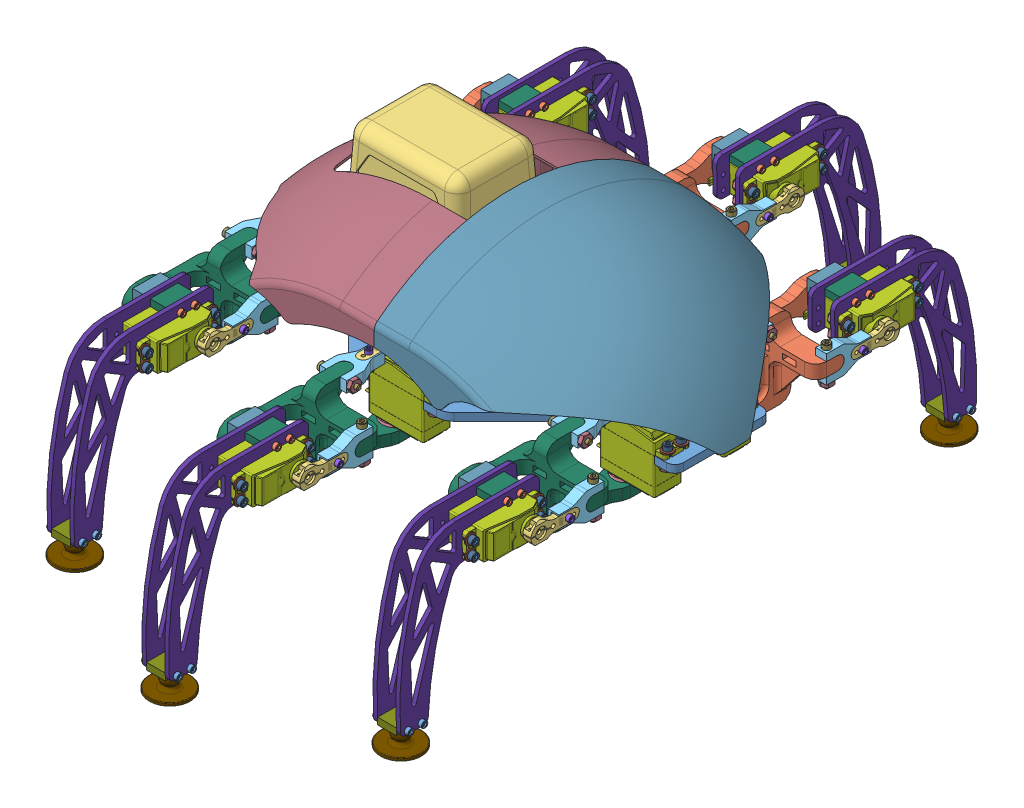
SolidWorks assembly Hexapod_(Small), configuration Défaut. Lengths in mm. (continued)
Components (placement in the parent): (continued)
- Foot+Femur_(Mirror)-8: Foot+Femur_(Mirror) [Défaut] at (-254.8 -28 0) x (0 0 1) z (-1 0 0) size (215.83 135.72 63.38)
  - Femur_(Mirror)-1: Femur_(Mirror) [Défaut] at origin size (137.38 61.64 60.79) (flexible)
    - Joint_(Femur_to_tibia)_(Mirror)-2: Joint_(Femur_to_tibia)_(Mirror) [Défaut] at (-66.2306 29.5 32.9516) x (0.999952 0 0.00979) z (-0.00979 0 0.999952) size (122 58.8 58.8)
    - Horn-4: Horn [Défaut] at (-10.2 48.8 30.1) x (-0.999952 0 -0.00979) z (0 1 0) size (35.39 15.87 6)
    - Bearing_mount_(Femur)-2: Bearing_mount_(Femur) [Default] at (2.5 22 30.1) x (1 0 0) z (0 -1 0) size (35.3 20.2 31)
    - Horn_attachment-4: Horn_attachment [Défaut] at (-38.1987 44.8 29.8259) x (0.999952 0 0.00979) z (0 1 0) size (33 20 8)
    - Bearing-4: Bearing [Default] at (-10.2 -6.7498 30.1) x (0.165905 0 -0.986142) z (0.986142 0 0.165905) size (13.87 4.75 13.87)
    - DS3225MG-4: DS3225MG [Default] at (-10.2 45.8 30.1) x (0 0 -1) z (0 1 0) size (57.25 20.4 45.91)
    - HX-SHCS 0.112-40x0.4375x0.4375-N-1: HX-SHCS 0.112-40x0.4375x0.4375-N [HX-SHCS 0.112-40x0.4375x0.4375-N] at (-30.199 51.6448 29.9042) x (0 -1 0) z (-0.508455 0 0.861089) size (13.96 4.65 4.65)
    - MSHXNUT 0.112-40-D-N-1: MSHXNUT 0.112-40-D-N [MSHXNUT 0.112-40-D-N] at (-30.199 40.8 29.9042) x (-0.491498 0 -0.870879) z (0 1 0) size (6.35 7.33 2.49)
    - HX-SHCS 0.138-32x0.5x0.5-N-1: HX-SHCS 0.138-32x0.5x0.5-N [HX-SHCS 0.138-32x0.5x0.5-N] at (-15.2 35.772 -4.7) x (0 -1 0) z (0.866025 0 -0.5) size (16.21 5.74 5.74)
    - Narrow FW 0.138-1: Narrow FW 0.138 [Narrow FW 0.138] at (-15.2 31.2 -4.7) x (0 -1 0) z (-0.829316 0 -0.55878) size (0.81 7.92 7.92)
    - HX-SHCS 0.138-32x0.5x0.5-N-2: HX-SHCS 0.138-32x0.5x0.5-N [HX-SHCS 0.138-32x0.5x0.5-N] at (-15.2 35.772 44.9) x (0 -1 0) z (0.866025 0 -0.5) size (16.21 5.74 5.74)
    - HX-SHCS 0.138-32x0.5x0.5-N-3: HX-SHCS 0.138-32x0.5x0.5-N [HX-SHCS 0.138-32x0.5x0.5-N] at (-5.2 35.772 -4.7) x (0 -1 0) z (0.866025 0 -0.5) size (16.21 5.74 5.74)
    - HX-SHCS 0.138-32x0.5x0.5-N-4: HX-SHCS 0.138-32x0.5x0.5-N [HX-SHCS 0.138-32x0.5x0.5-N] at (-5.2 35.772 44.9) x (0 -1 0) z (0.866025 0 -0.5) size (16.21 5.74 5.74)
    - Narrow FW 0.138-2: Narrow FW 0.138 [Narrow FW 0.138] at (-15.2 31.2 44.9) x (0 -1 0) z (-0.829316 0 -0.55878) size (0.81 7.92 7.92)
    - Narrow FW 0.138-3: Narrow FW 0.138 [Narrow FW 0.138] at (-5.2 31.2 -4.7) x (0 -1 0) z (-0.829316 0 -0.55878) size (0.81 7.92 7.92)
    - Narrow FW 0.138-4: Narrow FW 0.138 [Narrow FW 0.138] at (-5.2 31.2 44.9) x (0 -1 0) z (-0.829316 0 -0.55878) size (0.81 7.92 7.92)
    - HX-SHCS 0.138-32x1x1-N-1: HX-SHCS 0.138-32x1x1-N [HX-SHCS 0.138-32x1x1-N] at (-52.3302 44.8 43.1934) x (0.00979 0 -0.999952) z (-0.865984 0.5 -0.008479) size (28.91 5.74 5.74)
    - MSHXNUT 0.138-32-D-N-1: MSHXNUT 0.138-32-D-N [MSHXNUT 0.138-32-D-N] at (-52.0717 44.8 16.7938) x (0.865984 -0.5 0.008479) z (0.00979 0 -0.999952) size (7.92 9.15 2.9)
  - Foot_(Short)_(Mirror)-1: Foot_(Short)_(Mirror) [Défaut] at (-102.2988 19.1911 38.5987) x (0.999893 -0.010844 0.00979) z (-0.00979 0 0.999952) size (133.45 132 60.64) (flexible)
    - Horn_attachment-2: Horn_attachment [Défaut] at (17.8984 10.5036 -44.8) x (-0.999941 -0.010844 0) z (0 0 -1) size (33 20 8)
    - Bearing-2: Bearing [Default] at (-10.1 10.2 6.7498) x (0.20972 0.977761 0) z (-0.977761 0.20972 0) size (13.87 4.75 13.87)
    - Bearing_mount_(Foot)-2: Bearing_mount_(Foot) [Default] at (-10.1 22.9 -8.1) x (0 1 0) z (0 0 1) size (25.3 20.2 17.1)
    - Link-3: Link [Default] at (-10.1 22.9 -25) x (0 -1 0) z (0 0 1) size (5 20.2 13.9)
    - Horn-2: Horn [Défaut] at (-10.1 10.2 -48.8) x (0.999941 0.010844 0) z (0 0 -1) size (35.39 15.87 6)
    - Joint_(Foot_to_slipper)-4: Joint_(Foot_to_slipper) [Default] at (-82.4457 -87.5 -25) x (0 1 0) z (0 0 1) size (15 20.2 13.9)
    - Foot_(Short)-3: Foot_(Short) [Default] at (-21.5 14 -28) size (102.48 118 3)
    - DS3225MG-2: DS3225MG [Default] at (-10.1 10.2 -45.8) x (-1 0 0) z (0 0 -1) size (57.25 20.4 45.91)
    - Foot_(Short)-4: Foot_(Short) [Default] at (-21.5 14 -11.1) size (102.48 118 3)
    - Slipper-1: Slipper [Défaut] at (-82.4457 -102 -18.05) size (30 10.55 30)
    - HX-SHCS 0.112-40x0.4375x0.4375-N-1: HX-SHCS 0.112-40x0.4375x0.4375-N [HX-SHCS 0.112-40x0.4375x0.4375-N] at (9.8988 10.4169 -51.6448) x (0 0 1) z (0.509362 -0.860552 0) size (13.96 4.65 4.65)
    - MSHXNUT 0.112-40-D-N-1: MSHXNUT 0.112-40-D-N [MSHXNUT 0.112-40-D-N] at (9.8988 10.4169 -40.8) x (-0.509362 0.860552 0) z (0 0 -1) size (6.35 7.33 2.49)
    - HX-SHCS 0.112-40x0.875x0.875-N-1: HX-SHCS 0.112-40x0.875x0.875-N [HX-SHCS 0.112-40x0.875x0.875-N] at (-87.4457 -87.5 -30.8448) x (0 0 1) z (0 1 0) size (25.07 4.65 4.65)
    - MSHXNUT 0.112-40-D-N-2: MSHXNUT 0.112-40-D-N [MSHXNUT 0.112-40-D-N] at (-87.4457 -87.5 -8.1) x (-0.866025 -0.5 0) z (0 0 -1) size (6.35 7.33 2.49)
    - MSHXNUT 0.112-40-D-N-3: MSHXNUT 0.112-40-D-N [MSHXNUT 0.112-40-D-N] at (-77.4457 -87.5 -8.1) x (-0.866025 -0.5 0) z (0 0 -1) size (6.35 7.33 2.49)
    - HX-SHCS 0.112-40x0.875x0.875-N-2: HX-SHCS 0.112-40x0.875x0.875-N [HX-SHCS 0.112-40x0.875x0.875-N] at (-77.4457 -87.5 -30.8448) x (0 0 1) z (0 1 0) size (25.07 4.65 4.65)
    - HX-SHCS 0.112-40x1x0.75-N-3: HX-SHCS 0.112-40x1x0.75-N [HX-SHCS 0.112-40x1x0.75-N] at (-5.1 22.9 -30.8448) x (0 0 1) z (-0.866025 0.5 0) size (28.24 4.65 4.65)
    - HX-SHCS 0.112-40x1x0.75-N-4: HX-SHCS 0.112-40x1x0.75-N [HX-SHCS 0.112-40x1x0.75-N] at (-15.1 22.9 -30.8448) x (0 0 1) z (-0.866025 0.5 0) size (28.24 4.65 4.65)
    - HX-SHCS 0.138-32x0.5x0.5-N-1: HX-SHCS 0.138-32x0.5x0.5-N [HX-SHCS 0.138-32x0.5x0.5-N] at (-44.9 5.2 -35.772) x (0 0 1) z (-0.866025 0.5 0) size (16.21 5.74 5.74)
    - Narrow FW 0.138-1: Narrow FW 0.138 [Narrow FW 0.138] at (-44.9 5.2 -31.2) x (0 0 1) z (0.552023 0.833829 0) size (0.81 7.92 7.92)
    - MSHXNUT 0.138-32-D-N-1: MSHXNUT 0.138-32-D-N [MSHXNUT 0.138-32-D-N] at (-44.9 5.2 -25) x (-0.866025 -0.5 0) z (0 0 -1) size (7.92 9.15 2.9)
    - HX-SHCS 0.138-32x0.5x0.5-N-2: HX-SHCS 0.138-32x0.5x0.5-N [HX-SHCS 0.138-32x0.5x0.5-N] at (4.7 5.2 -35.772) x (0 0 1) z (-0.866025 0.5 0) size (16.21 5.74 5.74)
    - HX-SHCS 0.138-32x0.5x0.5-N-3: HX-SHCS 0.138-32x0.5x0.5-N [HX-SHCS 0.138-32x0.5x0.5-N] at (-44.9 15.2 -35.772) x (0 0 1) z (-0.866025 0.5 0) size (16.21 5.74 5.74)
    - HX-SHCS 0.138-32x0.5x0.5-N-4: HX-SHCS 0.138-32x0.5x0.5-N [HX-SHCS 0.138-32x0.5x0.5-N] at (4.7 15.2 -35.772) x (0 0 1) z (-0.866025 0.5 0) size (16.21 5.74 5.74)
    - Narrow FW 0.138-2: Narrow FW 0.138 [Narrow FW 0.138] at (4.7 5.2 -31.2) x (0 0 1) z (0.552023 0.833829 0) size (0.81 7.92 7.92)
    - Narrow FW 0.138-3: Narrow FW 0.138 [Narrow FW 0.138] at (-44.9 15.2 -31.2) x (0 0 1) z (0.552023 0.833829 0) size (0.81 7.92 7.92)
    - Narrow FW 0.138-4: Narrow FW 0.138 [Narrow FW 0.138] at (4.7 15.2 -31.2) x (0 0 1) z (0.552023 0.833829 0) size (0.81 7.92 7.92)
    - MSHXNUT 0.138-32-D-N-2: MSHXNUT 0.138-32-D-N [MSHXNUT 0.138-32-D-N] at (4.7 5.2 -25) x (-0.866025 -0.5 0) z (0 0 -1) size (7.92 9.15 2.9)
    - MSHXNUT 0.138-32-D-N-3: MSHXNUT 0.138-32-D-N [MSHXNUT 0.138-32-D-N] at (-44.9 15.2 -25) x (-0.866025 -0.5 0) z (0 0 -1) size (7.92 9.15 2.9)
    - MSHXNUT 0.138-32-D-N-4: MSHXNUT 0.138-32-D-N [MSHXNUT 0.138-32-D-N] at (4.7 15.2 -25) x (-0.866025 -0.5 0) z (0 0 -1) size (7.92 9.15 2.9)
  - HX-SHCS 0.138-32x1x1-N-1: HX-SHCS 0.138-32x1x1-N [HX-SHCS 0.138-32x1x1-N] at (-69.8506 43.0052 -5.8857) x (0 -1 0) z (0.861089 0 0.508455) size (28.91 5.74 5.74)
  - MSHXNUT 0.138-32-D-N-1: MSHXNUT 0.138-32-D-N [MSHXNUT 0.138-32-D-N] at (-69.8506 16.6044 -5.8857) x (0.00979 0 -0.999952) z (0 -1 0) size (7.92 9.15 2.9)
- Foot+Femur-1: Foot+Femur [Défaut] at (-254.8 -28 30.4) x (0 0 -1) z (1 0 0) size (214.66 136.49 62.17)
  - Femur-1: Femur [Défaut] at origin size (137.43 61.64 61.08) (flexible)
    - Joint_(Femur_to_tibia)-1: Joint_(Femur_to_tibia) [Défaut] at (-66.1066 29.5 -49.7675) x (0.999989 0 0.00478) z (-0.00478 0 0.999989) size (122 58.8 58.8)
    - Horn_attachment-3: Horn_attachment [Défaut] at (-38.1997 44.8 -30.2338) x (0.999989 0 0.00478) z (0 1 0) size (33 20 8)
    - Horn-3: Horn [Défaut] at (-10.2 48.8 -30.1) x (-0.999989 0 -0.00478) z (0 1 0) size (35.39 15.87 6)
    - DS3225MG-3: DS3225MG [Default] at (-10.2 45.8 -30.1) x (0 0 1) z (0 1 0) size (57.25 20.4 45.91)
    - Bearing_mount_(Femur)-1: Bearing_mount_(Femur) [Default] at (2.5 22 -30.1) x (1 0 0) z (0 -1 0) size (35.3 20.2 31)
    - Bearing-3: Bearing [Default] at (-10.2 -6.7498 -30.1) x (0.400474 0 0.916308) z (-0.916308 0 0.400474) size (13.87 4.75 13.87)
    - MSHXNUT 0.112-40-D-N-1: MSHXNUT 0.112-40-D-N [MSHXNUT 0.112-40-D-N] at (-30.1998 40.8 -30.1956) x (-0.495855 0 -0.868405) z (0 1 0) size (6.35 7.33 2.49)
    - HX-SHCS 0.112-40x0.4375x0.4375-N-1: HX-SHCS 0.112-40x0.4375x0.4375-N [HX-SHCS 0.112-40x0.4375x0.4375-N] at (-30.1998 51.6448 -30.1956) x (0 -1 0) z (-0.504134 0 0.863626) size (13.96 4.65 4.65)
    - Narrow FW 0.138-1: Narrow FW 0.138 [Narrow FW 0.138] at (-15.2 31.2 4.7) x (0 -1 0) z (-0.829316 0 -0.55878) size (0.81 7.92 7.92)
    - HX-SHCS 0.138-32x0.5x0.5-N-1: HX-SHCS 0.138-32x0.5x0.5-N [HX-SHCS 0.138-32x0.5x0.5-N] at (-15.2 35.772 4.7) x (0 -1 0) z (0.866025 0 -0.5) size (16.21 5.74 5.74)
    - Narrow FW 0.138-2: Narrow FW 0.138 [Narrow FW 0.138] at (-15.2 31.2 -44.9) x (0 -1 0) z (-0.829316 0 -0.55878) size (0.81 7.92 7.92)
    - Narrow FW 0.138-3: Narrow FW 0.138 [Narrow FW 0.138] at (-5.2 31.2 4.7) x (0 -1 0) z (-0.829316 0 -0.55878) size (0.81 7.92 7.92)
    - Narrow FW 0.138-4: Narrow FW 0.138 [Narrow FW 0.138] at (-5.2 31.2 -44.9) x (0 -1 0) z (-0.829316 0 -0.55878) size (0.81 7.92 7.92)
    - HX-SHCS 0.138-32x0.5x0.5-N-2: HX-SHCS 0.138-32x0.5x0.5-N [HX-SHCS 0.138-32x0.5x0.5-N] at (-15.2 35.772 -44.9) x (0 -1 0) z (0.866025 0 -0.5) size (16.21 5.74 5.74)
    - HX-SHCS 0.138-32x0.5x0.5-N-3: HX-SHCS 0.138-32x0.5x0.5-N [HX-SHCS 0.138-32x0.5x0.5-N] at (-5.2 35.772 4.7) x (0 -1 0) z (0.866025 0 -0.5) size (16.21 5.74 5.74)
    - HX-SHCS 0.138-32x0.5x0.5-N-4: HX-SHCS 0.138-32x0.5x0.5-N [HX-SHCS 0.138-32x0.5x0.5-N] at (-5.2 35.772 -44.9) x (0 -1 0) z (0.866025 0 -0.5) size (16.21 5.74 5.74)
    - MSHXNUT 0.138-32-D-N-1: MSHXNUT 0.138-32-D-N [MSHXNUT 0.138-32-D-N] at (-52.2612 44.8 -17.4053) x (-0.866016 -0.5 -0.004139) z (-0.00478 0 0.999989) size (7.92 9.15 2.9)
    - HX-SHCS 0.138-32x1x1-N-2: HX-SHCS 0.138-32x1x1-N [HX-SHCS 0.138-32x1x1-N] at (-52.135 44.8 -43.8058) x (-0.00478 0 0.999989) z (-0.866016 -0.5 -0.004139) size (28.91 5.74 5.74)
  - Foot_(Short)-15: Foot_(Short) [Défaut] at (-142.24 19.26 -40.1312) x (0.999988 0.00133 0.00478) z (-0.00478 0 0.999989) size (133.65 132.07 60.64) (flexible)
    - DS3225MG-1: DS3225MG [Default] at (30.1 10.2 45.8) x (-1 0 0) z (0 0 1) size (57.25 20.4 45.91)
    - Bearing-1: Bearing [Default] at (30.1 10.2 -6.7498) x (-0.564523 0.825417 0) z (0.825417 0.564523 0) size (13.87 4.75 13.87)
    - Bearing_mount_(Foot)-1: Bearing_mount_(Foot) [Default] at (30.1 22.9 8.1) x (0 1 0) z (0 0 -1) size (25.3 20.2 17.1)
    - Foot_(Short)-1: Foot_(Short) [Default] at (18.7 14 25) size (102.48 118 3)
    - Link-1: Link [Default] at (30.1 22.9 11.1) x (0 -1 0) z (0 0 1) size (5 20.2 13.9)
    - Foot_(Short)-2: Foot_(Short) [Default] at (18.7 14 8.1) size (102.48 118 3)
    - Joint_(Foot_to_slipper)-2: Joint_(Foot_to_slipper) [Default] at (-42.2457 -87.5 11.1) x (0 1 0) z (0 0 1) size (15 20.2 13.9)
    - Horn-1: Horn [Défaut] at (30.1 10.2 48.8) x (0.999999 -0.00133 0) z (0 0 1) size (35.39 15.87 6)
    - Horn_attachment-1: Horn_attachment [Défaut] at (58.1 10.1628 44.8) x (-0.999999 0.00133 0) z (0 0 1) size (33 20 8)
    - Slipper-1: Slipper [Défaut] at (-42.2774 -101.9999 18.0504) x (0.999844 -0.004527 -0.017101) z (0.017101 -0.000023 0.999854) size (30 10.55 30)
    - MSHXNUT 0.112-40-D-N-1: MSHXNUT 0.112-40-D-N [MSHXNUT 0.112-40-D-N] at (50.1 10.1734 40.8) x (0.999999 -0.00133 0) z (0 0 1) size (6.35 7.33 2.49)
    - HX-SHCS 0.112-40x0.4375x0.4375-N-1: HX-SHCS 0.112-40x0.4375x0.4375-N [HX-SHCS 0.112-40x0.4375x0.4375-N] at (50.1 10.1734 51.6448) x (0 0 -1) z (-0.498847 0.86669 0) size (13.96 4.65 4.65)
    - MSHXNUT 0.112-40-D-N-2: MSHXNUT 0.112-40-D-N [MSHXNUT 0.112-40-D-N] at (-47.2457 -87.5 8.1) x (0.866025 -0.5 0) z (0 0 1) size (6.35 7.33 2.49)
    - HX-SHCS 0.112-40x0.875x0.875-N-1: HX-SHCS 0.112-40x0.875x0.875-N [HX-SHCS 0.112-40x0.875x0.875-N] at (-47.2457 -87.5 30.8448) x (0 0 -1) z (0 1 0) size (25.07 4.65 4.65)
    - HX-SHCS 0.112-40x0.875x0.875-N-2: HX-SHCS 0.112-40x0.875x0.875-N [HX-SHCS 0.112-40x0.875x0.875-N] at (-37.2457 -87.5 30.8448) x (0 0 -1) z (0 1 0) size (25.07 4.65 4.65)
    - MSHXNUT 0.112-40-D-N-3: MSHXNUT 0.112-40-D-N [MSHXNUT 0.112-40-D-N] at (-37.2457 -87.5 8.1) x (0.866025 -0.5 0) z (0 0 1) size (6.35 7.33 2.49)
    - HX-SHCS 0.112-40x1x0.75-N-3: HX-SHCS 0.112-40x1x0.75-N [HX-SHCS 0.112-40x1x0.75-N] at (25.1 22.9 30.8448) x (0 0 -1) z (0 1 0) size (28.24 4.65 4.65)
    - HX-SHCS 0.112-40x1x0.75-N-4: HX-SHCS 0.112-40x1x0.75-N [HX-SHCS 0.112-40x1x0.75-N] at (35.1 22.9 30.8448) x (0 0 -1) z (0 1 0) size (28.24 4.65 4.65)
    - MSHXNUT 0.138-32-D-N-1: MSHXNUT 0.138-32-D-N [MSHXNUT 0.138-32-D-N] at (-4.7 5.2 25) x (0.866025 0.5 0) z (0 0 1) size (7.92 9.15 2.9)
    - Narrow FW 0.138-1: Narrow FW 0.138 [Narrow FW 0.138] at (-4.7 5.2 31.2) x (0 0 -1) z (-0.826778 0.562529 0) size (0.81 7.92 7.92)
    - HX-SHCS 0.138-32x0.5x0.5-N-1: HX-SHCS 0.138-32x0.5x0.5-N [HX-SHCS 0.138-32x0.5x0.5-N] at (-4.7 5.2 35.772) x (0 0 -1) z (0.866025 0.5 0) size (16.21 5.74 5.74)
    - MSHXNUT 0.138-32-D-N-2: MSHXNUT 0.138-32-D-N [MSHXNUT 0.138-32-D-N] at (44.9 5.2 25) x (0.866025 0.5 0) z (0 0 1) size (7.92 9.15 2.9)
    - MSHXNUT 0.138-32-D-N-3: MSHXNUT 0.138-32-D-N [MSHXNUT 0.138-32-D-N] at (-4.7 15.2 25) x (0.866025 0.5 0) z (0 0 1) size (7.92 9.15 2.9)
    - MSHXNUT 0.138-32-D-N-4: MSHXNUT 0.138-32-D-N [MSHXNUT 0.138-32-D-N] at (44.9 15.2 25) x (0.866025 0.5 0) z (0 0 1) size (7.92 9.15 2.9)
    - Narrow FW 0.138-2: Narrow FW 0.138 [Narrow FW 0.138] at (44.9 5.2 31.2) x (0 0 -1) z (-0.826778 0.562529 0) size (0.81 7.92 7.92)
    - Narrow FW 0.138-3: Narrow FW 0.138 [Narrow FW 0.138] at (-4.7 15.2 31.2) x (0 0 -1) z (-0.826778 0.562529 0) size (0.81 7.92 7.92)
    - Narrow FW 0.138-4: Narrow FW 0.138 [Narrow FW 0.138] at (44.9 15.2 31.2) x (0 0 -1) z (-0.826778 0.562529 0) size (0.81 7.92 7.92)
    - HX-SHCS 0.138-32x0.5x0.5-N-2: HX-SHCS 0.138-32x0.5x0.5-N [HX-SHCS 0.138-32x0.5x0.5-N] at (44.9 5.2 35.772) x (0 0 -1) z (0.866025 0.5 0) size (16.21 5.74 5.74)
    - HX-SHCS 0.138-32x0.5x0.5-N-3: HX-SHCS 0.138-32x0.5x0.5-N [HX-SHCS 0.138-32x0.5x0.5-N] at (-4.7 15.2 35.772) x (0 0 -1) z (0.866025 0.5 0) size (16.21 5.74 5.74)
    - HX-SHCS 0.138-32x0.5x0.5-N-4: HX-SHCS 0.138-32x0.5x0.5-N [HX-SHCS 0.138-32x0.5x0.5-N] at (44.9 15.2 35.772) x (0 0 -1) z (0.866025 0.5 0) size (16.21 5.74 5.74)
  - MSHXNUT 0.138-32-D-N-1: MSHXNUT 0.138-32-D-N [MSHXNUT 0.138-32-D-N] at (-70.3685 16.6044 5.0128) x (-0.863626 0 -0.504134) z (0 -1 0) size (7.92 9.15 2.9)
  - HX-SHCS 0.138-32x1x1-N-1: HX-SHCS 0.138-32x1x1-N [HX-SHCS 0.138-32x1x1-N] at (-70.3685 43.0052 5.0128) x (0 -1 0) z (0.00478 0 -0.999989) size (28.91 5.74 5.74)
- Foot+Femur-3: Foot+Femur [Défaut] at (-134.8 -28 80.6) x (0 0 -1) z (1 0 0) size (214.66 136.49 62.17)
  - Femur-1: Femur [Défaut] at origin size (137.43 61.64 61.08) (flexible)
    - Joint_(Femur_to_tibia)-1: Joint_(Femur_to_tibia) [Défaut] at (-66.1066 29.5 -49.7675) x (0.999989 0 0.00478) z (-0.00478 0 0.999989) size (122 58.8 58.8)
    - Horn_attachment-3: Horn_attachment [Défaut] at (-38.1997 44.8 -30.2338) x (0.999989 0 0.00478) z (0 1 0) size (33 20 8)
    - Horn-3: Horn [Défaut] at (-10.2 48.8 -30.1) x (-0.999989 0 -0.00478) z (0 1 0) size (35.39 15.87 6)
    - DS3225MG-3: DS3225MG [Default] at (-10.2 45.8 -30.1) x (0 0 1) z (0 1 0) size (57.25 20.4 45.91)
    - Bearing_mount_(Femur)-1: Bearing_mount_(Femur) [Default] at (2.5 22 -30.1) x (1 0 0) z (0 -1 0) size (35.3 20.2 31)
    - Bearing-3: Bearing [Default] at (-10.2 -6.7498 -30.1) x (0.400474 0 0.916308) z (-0.916308 0 0.400474) size (13.87 4.75 13.87)
    - MSHXNUT 0.112-40-D-N-1: MSHXNUT 0.112-40-D-N [MSHXNUT 0.112-40-D-N] at (-30.1998 40.8 -30.1956) x (-0.495855 0 -0.868405) z (0 1 0) size (6.35 7.33 2.49)
    - HX-SHCS 0.112-40x0.4375x0.4375-N-1: HX-SHCS 0.112-40x0.4375x0.4375-N [HX-SHCS 0.112-40x0.4375x0.4375-N] at (-30.1998 51.6448 -30.1956) x (0 -1 0) z (-0.504134 0 0.863626) size (13.96 4.65 4.65)
    - Narrow FW 0.138-1: Narrow FW 0.138 [Narrow FW 0.138] at (-15.2 31.2 4.7) x (0 -1 0) z (-0.829316 0 -0.55878) size (0.81 7.92 7.92)
    - HX-SHCS 0.138-32x0.5x0.5-N-1: HX-SHCS 0.138-32x0.5x0.5-N [HX-SHCS 0.138-32x0.5x0.5-N] at (-15.2 35.772 4.7) x (0 -1 0) z (0.866025 0 -0.5) size (16.21 5.74 5.74)
    - Narrow FW 0.138-2: Narrow FW 0.138 [Narrow FW 0.138] at (-15.2 31.2 -44.9) x (0 -1 0) z (-0.829316 0 -0.55878) size (0.81 7.92 7.92)
    - Narrow FW 0.138-3: Narrow FW 0.138 [Narrow FW 0.138] at (-5.2 31.2 4.7) x (0 -1 0) z (-0.829316 0 -0.55878) size (0.81 7.92 7.92)
    - Narrow FW 0.138-4: Narrow FW 0.138 [Narrow FW 0.138] at (-5.2 31.2 -44.9) x (0 -1 0) z (-0.829316 0 -0.55878) size (0.81 7.92 7.92)
    - HX-SHCS 0.138-32x0.5x0.5-N-2: HX-SHCS 0.138-32x0.5x0.5-N [HX-SHCS 0.138-32x0.5x0.5-N] at (-15.2 35.772 -44.9) x (0 -1 0) z (0.866025 0 -0.5) size (16.21 5.74 5.74)
    - HX-SHCS 0.138-32x0.5x0.5-N-3: HX-SHCS 0.138-32x0.5x0.5-N [HX-SHCS 0.138-32x0.5x0.5-N] at (-5.2 35.772 4.7) x (0 -1 0) z (0.866025 0 -0.5) size (16.21 5.74 5.74)
    - HX-SHCS 0.138-32x0.5x0.5-N-4: HX-SHCS 0.138-32x0.5x0.5-N [HX-SHCS 0.138-32x0.5x0.5-N] at (-5.2 35.772 -44.9) x (0 -1 0) z (0.866025 0 -0.5) size (16.21 5.74 5.74)
    - MSHXNUT 0.138-32-D-N-1: MSHXNUT 0.138-32-D-N [MSHXNUT 0.138-32-D-N] at (-52.2612 44.8 -17.4053) x (-0.866016 -0.5 -0.004139) z (-0.00478 0 0.999989) size (7.92 9.15 2.9)
    - HX-SHCS 0.138-32x1x1-N-2: HX-SHCS 0.138-32x1x1-N [HX-SHCS 0.138-32x1x1-N] at (-52.135 44.8 -43.8058) x (-0.00478 0 0.999989) z (-0.866016 -0.5 -0.004139) size (28.91 5.74 5.74)
  - Foot_(Short)-15: Foot_(Short) [Défaut] at (-142.24 19.26 -40.1312) x (0.999988 0.00133 0.00478) z (-0.00478 0 0.999989) size (133.65 132.07 60.64) (flexible)
    - DS3225MG-1: DS3225MG [Default] at (30.1 10.2 45.8) x (-1 0 0) z (0 0 1) size (57.25 20.4 45.91)
    - Bearing-1: Bearing [Default] at (30.1 10.2 -6.7498) x (-0.564523 0.825417 0) z (0.825417 0.564523 0) size (13.87 4.75 13.87)
    - Bearing_mount_(Foot)-1: Bearing_mount_(Foot) [Default] at (30.1 22.9 8.1) x (0 1 0) z (0 0 -1) size (25.3 20.2 17.1)
    - Foot_(Short)-1: Foot_(Short) [Default] at (18.7 14 25) size (102.48 118 3)
    - Link-1: Link [Default] at (30.1 22.9 11.1) x (0 -1 0) z (0 0 1) size (5 20.2 13.9)
    - Foot_(Short)-2: Foot_(Short) [Default] at (18.7 14 8.1) size (102.48 118 3)
    - Joint_(Foot_to_slipper)-2: Joint_(Foot_to_slipper) [Default] at (-42.2457 -87.5 11.1) x (0 1 0) z (0 0 1) size (15 20.2 13.9)
    - Horn-1: Horn [Défaut] at (30.1 10.2 48.8) x (0.999999 -0.00133 0) z (0 0 1) size (35.39 15.87 6)
    - Horn_attachment-1: Horn_attachment [Défaut] at (58.1 10.1628 44.8) x (-0.999999 0.00133 0) z (0 0 1) size (33 20 8)
    - Slipper-1: Slipper [Défaut] at (-42.2774 -101.9999 18.0504) x (0.999844 -0.004527 -0.017101) z (0.017101 -0.000023 0.999854) size (30 10.55 30)
    - MSHXNUT 0.112-40-D-N-1: MSHXNUT 0.112-40-D-N [MSHXNUT 0.112-40-D-N] at (50.1 10.1734 40.8) x (0.999999 -0.00133 0) z (0 0 1) size (6.35 7.33 2.49)
    - HX-SHCS 0.112-40x0.4375x0.4375-N-1: HX-SHCS 0.112-40x0.4375x0.4375-N [HX-SHCS 0.112-40x0.4375x0.4375-N] at (50.1 10.1734 51.6448) x (0 0 -1) z (-0.498847 0.86669 0) size (13.96 4.65 4.65)
    - MSHXNUT 0.112-40-D-N-2: MSHXNUT 0.112-40-D-N [MSHXNUT 0.112-40-D-N] at (-47.2457 -87.5 8.1) x (0.866025 -0.5 0) z (0 0 1) size (6.35 7.33 2.49)
    - HX-SHCS 0.112-40x0.875x0.875-N-1: HX-SHCS 0.112-40x0.875x0.875-N [HX-SHCS 0.112-40x0.875x0.875-N] at (-47.2457 -87.5 30.8448) x (0 0 -1) z (0 1 0) size (25.07 4.65 4.65)
    - HX-SHCS 0.112-40x0.875x0.875-N-2: HX-SHCS 0.112-40x0.875x0.875-N [HX-SHCS 0.112-40x0.875x0.875-N] at (-37.2457 -87.5 30.8448) x (0 0 -1) z (0 1 0) size (25.07 4.65 4.65)
    - MSHXNUT 0.112-40-D-N-3: MSHXNUT 0.112-40-D-N [MSHXNUT 0.112-40-D-N] at (-37.2457 -87.5 8.1) x (0.866025 -0.5 0) z (0 0 1) size (6.35 7.33 2.49)
    - HX-SHCS 0.112-40x1x0.75-N-3: HX-SHCS 0.112-40x1x0.75-N [HX-SHCS 0.112-40x1x0.75-N] at (25.1 22.9 30.8448) x (0 0 -1) z (0 1 0) size (28.24 4.65 4.65)
    - HX-SHCS 0.112-40x1x0.75-N-4: HX-SHCS 0.112-40x1x0.75-N [HX-SHCS 0.112-40x1x0.75-N] at (35.1 22.9 30.8448) x (0 0 -1) z (0 1 0) size (28.24 4.65 4.65)
    - MSHXNUT 0.138-32-D-N-1: MSHXNUT 0.138-32-D-N [MSHXNUT 0.138-32-D-N] at (-4.7 5.2 25) x (0.866025 0.5 0) z (0 0 1) size (7.92 9.15 2.9)
    - Narrow FW 0.138-1: Narrow FW 0.138 [Narrow FW 0.138] at (-4.7 5.2 31.2) x (0 0 -1) z (-0.826778 0.562529 0) size (0.81 7.92 7.92)
    - HX-SHCS 0.138-32x0.5x0.5-N-1: HX-SHCS 0.138-32x0.5x0.5-N [HX-SHCS 0.138-32x0.5x0.5-N] at (-4.7 5.2 35.772) x (0 0 -1) z (0.866025 0.5 0) size (16.21 5.74 5.74)
    - MSHXNUT 0.138-32-D-N-2: MSHXNUT 0.138-32-D-N [MSHXNUT 0.138-32-D-N] at (44.9 5.2 25) x (0.866025 0.5 0) z (0 0 1) size (7.92 9.15 2.9)
    - MSHXNUT 0.138-32-D-N-3: MSHXNUT 0.138-32-D-N [MSHXNUT 0.138-32-D-N] at (-4.7 15.2 25) x (0.866025 0.5 0) z (0 0 1) size (7.92 9.15 2.9)
    - MSHXNUT 0.138-32-D-N-4: MSHXNUT 0.138-32-D-N [MSHXNUT 0.138-32-D-N] at (44.9 15.2 25) x (0.866025 0.5 0) z (0 0 1) size (7.92 9.15 2.9)
    - Narrow FW 0.138-2: Narrow FW 0.138 [Narrow FW 0.138] at (44.9 5.2 31.2) x (0 0 -1) z (-0.826778 0.562529 0) size (0.81 7.92 7.92)
    - Narrow FW 0.138-3: Narrow FW 0.138 [Narrow FW 0.138] at (-4.7 15.2 31.2) x (0 0 -1) z (-0.826778 0.562529 0) size (0.81 7.92 7.92)
    - Narrow FW 0.138-4: Narrow FW 0.138 [Narrow FW 0.138] at (44.9 15.2 31.2) x (0 0 -1) z (-0.826778 0.562529 0) size (0.81 7.92 7.92)
    - HX-SHCS 0.138-32x0.5x0.5-N-2: HX-SHCS 0.138-32x0.5x0.5-N [HX-SHCS 0.138-32x0.5x0.5-N] at (44.9 5.2 35.772) x (0 0 -1) z (0.866025 0.5 0) size (16.21 5.74 5.74)
    - HX-SHCS 0.138-32x0.5x0.5-N-3: HX-SHCS 0.138-32x0.5x0.5-N [HX-SHCS 0.138-32x0.5x0.5-N] at (-4.7 15.2 35.772) x (0 0 -1) z (0.866025 0.5 0) size (16.21 5.74 5.74)
    - HX-SHCS 0.138-32x0.5x0.5-N-4: HX-SHCS 0.138-32x0.5x0.5-N [HX-SHCS 0.138-32x0.5x0.5-N] at (44.9 15.2 35.772) x (0 0 -1) z (0.866025 0.5 0) size (16.21 5.74 5.74)
  - MSHXNUT 0.138-32-D-N-1: MSHXNUT 0.138-32-D-N [MSHXNUT 0.138-32-D-N] at (-70.3685 16.6044 5.0128) x (-0.863626 0 -0.504134) z (0 -1 0) size (7.92 9.15 2.9)
  - HX-SHCS 0.138-32x1x1-N-1: HX-SHCS 0.138-32x1x1-N [HX-SHCS 0.138-32x1x1-N] at (-70.3685 43.0052 5.0128) x (0 -1 0) z (0.00478 0 -0.999989) size (28.91 5.74 5.74)
- Foot+Femur-4: Foot+Femur [Défaut] at (-14.8 -28 30.6) x (0 0 -1) z (1 0 0) size (214.66 136.49 62.17)
  - Femur-1: Femur [Défaut] at origin size (137.43 61.64 61.08) (flexible)
    - Joint_(Femur_to_tibia)-1: Joint_(Femur_to_tibia) [Défaut] at (-66.1066 29.5 -49.7675) x (0.999989 0 0.00478) z (-0.00478 0 0.999989) size (122 58.8 58.8)
    - Horn_attachment-3: Horn_attachment [Défaut] at (-38.1997 44.8 -30.2338) x (0.999989 0 0.00478) z (0 1 0) size (33 20 8)
    - Horn-3: Horn [Défaut] at (-10.2 48.8 -30.1) x (-0.999989 0 -0.00478) z (0 1 0) size (35.39 15.87 6)
    - DS3225MG-3: DS3225MG [Default] at (-10.2 45.8 -30.1) x (0 0 1) z (0 1 0) size (57.25 20.4 45.91)
    - Bearing_mount_(Femur)-1: Bearing_mount_(Femur) [Default] at (2.5 22 -30.1) x (1 0 0) z (0 -1 0) size (35.3 20.2 31)
    - Bearing-3: Bearing [Default] at (-10.2 -6.7498 -30.1) x (0.400474 0 0.916308) z (-0.916308 0 0.400474) size (13.87 4.75 13.87)
    - MSHXNUT 0.112-40-D-N-1: MSHXNUT 0.112-40-D-N [MSHXNUT 0.112-40-D-N] at (-30.1998 40.8 -30.1956) x (-0.495855 0 -0.868405) z (0 1 0) size (6.35 7.33 2.49)
    - HX-SHCS 0.112-40x0.4375x0.4375-N-1: HX-SHCS 0.112-40x0.4375x0.4375-N [HX-SHCS 0.112-40x0.4375x0.4375-N] at (-30.1998 51.6448 -30.1956) x (0 -1 0) z (-0.504134 0 0.863626) size (13.96 4.65 4.65)
    - Narrow FW 0.138-1: Narrow FW 0.138 [Narrow FW 0.138] at (-15.2 31.2 4.7) x (0 -1 0) z (-0.829316 0 -0.55878) size (0.81 7.92 7.92)
    - HX-SHCS 0.138-32x0.5x0.5-N-1: HX-SHCS 0.138-32x0.5x0.5-N [HX-SHCS 0.138-32x0.5x0.5-N] at (-15.2 35.772 4.7) x (0 -1 0) z (0.866025 0 -0.5) size (16.21 5.74 5.74)
    - Narrow FW 0.138-2: Narrow FW 0.138 [Narrow FW 0.138] at (-15.2 31.2 -44.9) x (0 -1 0) z (-0.829316 0 -0.55878) size (0.81 7.92 7.92)
    - Narrow FW 0.138-3: Narrow FW 0.138 [Narrow FW 0.138] at (-5.2 31.2 4.7) x (0 -1 0) z (-0.829316 0 -0.55878) size (0.81 7.92 7.92)
    - Narrow FW 0.138-4: Narrow FW 0.138 [Narrow FW 0.138] at (-5.2 31.2 -44.9) x (0 -1 0) z (-0.829316 0 -0.55878) size (0.81 7.92 7.92)
    - HX-SHCS 0.138-32x0.5x0.5-N-2: HX-SHCS 0.138-32x0.5x0.5-N [HX-SHCS 0.138-32x0.5x0.5-N] at (-15.2 35.772 -44.9) x (0 -1 0) z (0.866025 0 -0.5) size (16.21 5.74 5.74)
    - HX-SHCS 0.138-32x0.5x0.5-N-3: HX-SHCS 0.138-32x0.5x0.5-N [HX-SHCS 0.138-32x0.5x0.5-N] at (-5.2 35.772 4.7) x (0 -1 0) z (0.866025 0 -0.5) size (16.21 5.74 5.74)
    - HX-SHCS 0.138-32x0.5x0.5-N-4: HX-SHCS 0.138-32x0.5x0.5-N [HX-SHCS 0.138-32x0.5x0.5-N] at (-5.2 35.772 -44.9) x (0 -1 0) z (0.866025 0 -0.5) size (16.21 5.74 5.74)
    - MSHXNUT 0.138-32-D-N-1: MSHXNUT 0.138-32-D-N [MSHXNUT 0.138-32-D-N] at (-52.2612 44.8 -17.4053) x (-0.866016 -0.5 -0.004139) z (-0.00478 0 0.999989) size (7.92 9.15 2.9)
    - HX-SHCS 0.138-32x1x1-N-2: HX-SHCS 0.138-32x1x1-N [HX-SHCS 0.138-32x1x1-N] at (-52.135 44.8 -43.8058) x (-0.00478 0 0.999989) z (-0.866016 -0.5 -0.004139) size (28.91 5.74 5.74)
  - Foot_(Short)-15: Foot_(Short) [Défaut] at (-142.24 19.26 -40.1312) x (0.999988 0.00133 0.00478) z (-0.00478 0 0.999989) size (133.65 132.07 60.64) (flexible)
    - DS3225MG-1: DS3225MG [Default] at (30.1 10.2 45.8) x (-1 0 0) z (0 0 1) size (57.25 20.4 45.91)
    - Bearing-1: Bearing [Default] at (30.1 10.2 -6.7498) x (-0.564523 0.825417 0) z (0.825417 0.564523 0) size (13.87 4.75 13.87)
    - Bearing_mount_(Foot)-1: Bearing_mount_(Foot) [Default] at (30.1 22.9 8.1) x (0 1 0) z (0 0 -1) size (25.3 20.2 17.1)
    - Foot_(Short)-1: Foot_(Short) [Default] at (18.7 14 25) size (102.48 118 3)
    - Link-1: Link [Default] at (30.1 22.9 11.1) x (0 -1 0) z (0 0 1) size (5 20.2 13.9)
    - Foot_(Short)-2: Foot_(Short) [Default] at (18.7 14 8.1) size (102.48 118 3)
    - Joint_(Foot_to_slipper)-2: Joint_(Foot_to_slipper) [Default] at (-42.2457 -87.5 11.1) x (0 1 0) z (0 0 1) size (15 20.2 13.9)
    - Horn-1: Horn [Défaut] at (30.1 10.2 48.8) x (0.999999 -0.00133 0) z (0 0 1) size (35.39 15.87 6)
    - Horn_attachment-1: Horn_attachment [Défaut] at (58.1 10.1628 44.8) x (-0.999999 0.00133 0) z (0 0 1) size (33 20 8)
    - Slipper-1: Slipper [Défaut] at (-42.2774 -101.9999 18.0504) x (0.999844 -0.004527 -0.017101) z (0.017101 -0.000023 0.999854) size (30 10.55 30)
    - MSHXNUT 0.112-40-D-N-1: MSHXNUT 0.112-40-D-N [MSHXNUT 0.112-40-D-N] at (50.1 10.1734 40.8) x (0.999999 -0.00133 0) z (0 0 1) size (6.35 7.33 2.49)
    - HX-SHCS 0.112-40x0.4375x0.4375-N-1: HX-SHCS 0.112-40x0.4375x0.4375-N [HX-SHCS 0.112-40x0.4375x0.4375-N] at (50.1 10.1734 51.6448) x (0 0 -1) z (-0.498847 0.86669 0) size (13.96 4.65 4.65)
    - MSHXNUT 0.112-40-D-N-2: MSHXNUT 0.112-40-D-N [MSHXNUT 0.112-40-D-N] at (-47.2457 -87.5 8.1) x (0.866025 -0.5 0) z (0 0 1) size (6.35 7.33 2.49)
    - HX-SHCS 0.112-40x0.875x0.875-N-1: HX-SHCS 0.112-40x0.875x0.875-N [HX-SHCS 0.112-40x0.875x0.875-N] at (-47.2457 -87.5 30.8448) x (0 0 -1) z (0 1 0) size (25.07 4.65 4.65)
    - HX-SHCS 0.112-40x0.875x0.875-N-2: HX-SHCS 0.112-40x0.875x0.875-N [HX-SHCS 0.112-40x0.875x0.875-N] at (-37.2457 -87.5 30.8448) x (0 0 -1) z (0 1 0) size (25.07 4.65 4.65)
    - MSHXNUT 0.112-40-D-N-3: MSHXNUT 0.112-40-D-N [MSHXNUT 0.112-40-D-N] at (-37.2457 -87.5 8.1) x (0.866025 -0.5 0) z (0 0 1) size (6.35 7.33 2.49)
    - HX-SHCS 0.112-40x1x0.75-N-3: HX-SHCS 0.112-40x1x0.75-N [HX-SHCS 0.112-40x1x0.75-N] at (25.1 22.9 30.8448) x (0 0 -1) z (0 1 0) size (28.24 4.65 4.65)
    - HX-SHCS 0.112-40x1x0.75-N-4: HX-SHCS 0.112-40x1x0.75-N [HX-SHCS 0.112-40x1x0.75-N] at (35.1 22.9 30.8448) x (0 0 -1) z (0 1 0) size (28.24 4.65 4.65)
    - MSHXNUT 0.138-32-D-N-1: MSHXNUT 0.138-32-D-N [MSHXNUT 0.138-32-D-N] at (-4.7 5.2 25) x (0.866025 0.5 0) z (0 0 1) size (7.92 9.15 2.9)
    - Narrow FW 0.138-1: Narrow FW 0.138 [Narrow FW 0.138] at (-4.7 5.2 31.2) x (0 0 -1) z (-0.826778 0.562529 0) size (0.81 7.92 7.92)
    - HX-SHCS 0.138-32x0.5x0.5-N-1: HX-SHCS 0.138-32x0.5x0.5-N [HX-SHCS 0.138-32x0.5x0.5-N] at (-4.7 5.2 35.772) x (0 0 -1) z (0.866025 0.5 0) size (16.21 5.74 5.74)
    - MSHXNUT 0.138-32-D-N-2: MSHXNUT 0.138-32-D-N [MSHXNUT 0.138-32-D-N] at (44.9 5.2 25) x (0.866025 0.5 0) z (0 0 1) size (7.92 9.15 2.9)
    - MSHXNUT 0.138-32-D-N-3: MSHXNUT 0.138-32-D-N [MSHXNUT 0.138-32-D-N] at (-4.7 15.2 25) x (0.866025 0.5 0) z (0 0 1) size (7.92 9.15 2.9)
    - MSHXNUT 0.138-32-D-N-4: MSHXNUT 0.138-32-D-N [MSHXNUT 0.138-32-D-N] at (44.9 15.2 25) x (0.866025 0.5 0) z (0 0 1) size (7.92 9.15 2.9)
    - Narrow FW 0.138-2: Narrow FW 0.138 [Narrow FW 0.138] at (44.9 5.2 31.2) x (0 0 -1) z (-0.826778 0.562529 0) size (0.81 7.92 7.92)
    - Narrow FW 0.138-3: Narrow FW 0.138 [Narrow FW 0.138] at (-4.7 15.2 31.2) x (0 0 -1) z (-0.826778 0.562529 0) size (0.81 7.92 7.92)
    - Narrow FW 0.138-4: Narrow FW 0.138 [Narrow FW 0.138] at (44.9 15.2 31.2) x (0 0 -1) z (-0.826778 0.562529 0) size (0.81 7.92 7.92)
    - HX-SHCS 0.138-32x0.5x0.5-N-2: HX-SHCS 0.138-32x0.5x0.5-N [HX-SHCS 0.138-32x0.5x0.5-N] at (44.9 5.2 35.772) x (0 0 -1) z (0.866025 0.5 0) size (16.21 5.74 5.74)
    - HX-SHCS 0.138-32x0.5x0.5-N-3: HX-SHCS 0.138-32x0.5x0.5-N [HX-SHCS 0.138-32x0.5x0.5-N] at (-4.7 15.2 35.772) x (0 0 -1) z (0.866025 0.5 0) size (16.21 5.74 5.74)
    - HX-SHCS 0.138-32x0.5x0.5-N-4: HX-SHCS 0.138-32x0.5x0.5-N [HX-SHCS 0.138-32x0.5x0.5-N] at (44.9 15.2 35.772) x (0 0 -1) z (0.866025 0.5 0) size (16.21 5.74 5.74)
  - MSHXNUT 0.138-32-D-N-1: MSHXNUT 0.138-32-D-N [MSHXNUT 0.138-32-D-N] at (-70.3685 16.6044 5.0128) x (-0.863626 0 -0.504134) z (0 -1 0) size (7.92 9.15 2.9)
  - HX-SHCS 0.138-32x1x1-N-1: HX-SHCS 0.138-32x1x1-N [HX-SHCS 0.138-32x1x1-N] at (-70.3685 43.0052 5.0128) x (0 -1 0) z (0.00478 0 -0.999989) size (28.91 5.74 5.74)
